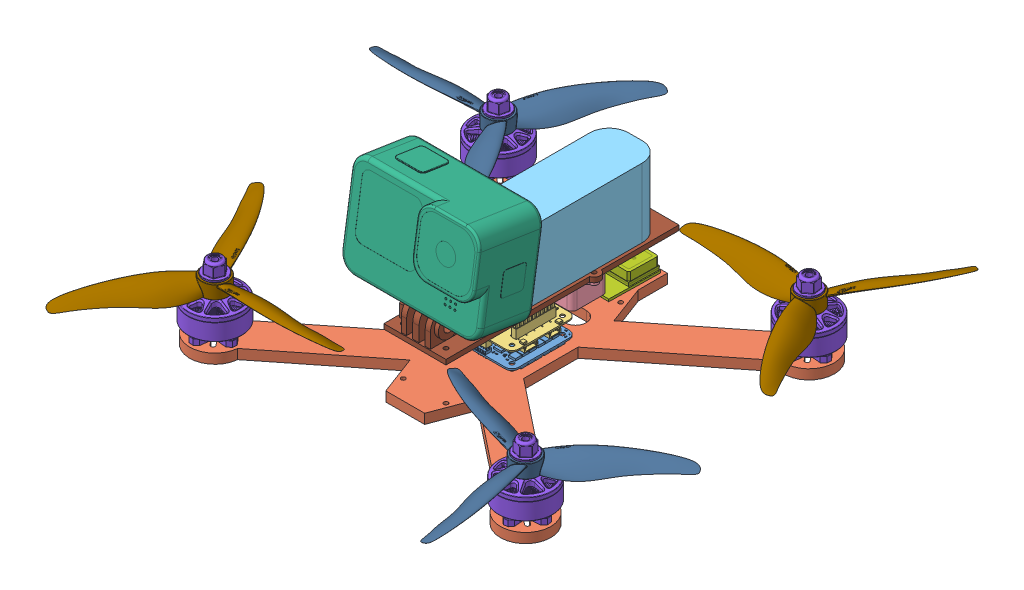
SolidWorks assembly Quad_assem, configuration Default. Lengths in mm.
Overall size (310.74 97.21 293.5).
16 component instances, 11 part files, 39 mates.
Components (placement in the parent):
- 4in1_ESC-1: 4in1_ESC [Default] at (-19.4317 7.836 116.374) x (-1 0 0) z (0 1 0) size (33 33 7.6)
- Quad-1: Quad [Default] at (-19.4317 0 116.374) x (-1 0 0) z (0 0 -1) size (186 5 172)
- FlightController.step-1: FlightController.step [Default] at (-19.4317 15.9597 116.374) x (-1 0 0) z (0 1 0) size (33 33 15.78)
- ToF-1: ToF [Default] at (-19.4317 27 89.374) x (1 0 0) z (0 0 -1) size (34.5 13.5 18.5)
- Battery-1: Battery [Default] at (-5 47.25 90.057) x (0 0 1) z (-1 0 0) size (72.6 35.5 27)
- GoPro Hero 9-1: GoPro Hero 9 [Default] at (-54.98 91.6448 135.3186) x (1 0 0) z (0 -0.98853 0.151026) size (72.1 33.6 50.5)
- GPS_sam-m8q-2: GPS_sam-m8q [Default] at (-27.0693 6.25 48.1086) x (0.999848 0 0.017452) z (-0.017452 0 0.999848) size (16.15 7.55 26.25)
- DYS SF2207 Motor.step-1: DYS SF2207 Motor.step [Default] at (60.5683 5 189.374) x (0.969016 0 -0.246999) z (0.246999 0 0.969016) size (27.7 33.34 27.7)
- DYS SF2207 Motor.step-2: DYS SF2207 Motor.step [Default] at (60.5683 5 43.374) x (0.997185 0 -0.074979) z (0.074979 0 0.997185) size (27.7 33.34 27.7)
- DYS SF2207 Motor.step-3: DYS SF2207 Motor.step [Default] at (-99.4317 5 43.374) x (0.246999 0 0.969016) z (-0.969016 0 0.246999) size (27.7 33.34 27.7)
- DYS SF2207 Motor.step-4: DYS SF2207 Motor.step [Default] at (-99.4317 5 189.374) x (0.074979 0 0.997185) z (-0.997185 0 0.074979) size (27.7 33.34 27.7)
- 50 Prop CW-1: 50 Prop CW [Default] at (60.5683 24.2 43.374) x (0.500095 0 -0.865971) z (0.865971 0 0.500095) size (98.6 8.5 111.89)
- 50 Prop CCW-1: 50 Prop CCW [Default] at (140.3677 27.725 231.543) x (-0.75515 0 0.655552) z (-0.655552 0 -0.75515) size (98.59 8.5 111.89)
- 50 Prop CCW-2: 50 Prop CCW [Default] at (-9.7231 27.725 53.3005) x (-0.461735 0 0.887018) z (-0.887018 0 -0.461735) size (98.59 8.5 111.89)
- 50 Prop CW-2: 50 Prop CW [Default] at (-99.4317 24.2 189.374) size (98.6 8.5 111.89)
- Quad Top-1: Quad Top [Default] at (-19.4317 27 116.374) x (-1 0 0) z (0 0 -1) size (36.7 17.5 120)
Mates (geometry in assembly coordinates):
- Concentric3: concentric aligned: circle of 4in1_ESC-1; circle of FlightController.step-1
- Concentric4: concentric aligned: circle of 4in1_ESC-1; circle of FlightController.step-1
- Distance3: distance = 7.5 mm anti-aligned: plane of 4in1_ESC-1 through (-2.9317 7.836 103.374) normal (0 1 0); plane of FlightController.step-1 through (-2.9317 15.336 103.374) normal (0 -1 0)
- Distance6: distance = 5 mm aligned: plane of Battery-1 through (-5 47.25 90.057) normal (1 0 0)
- Distance7: distance = 55 mm anti-aligned: plane of GoPro Hero 9-1 through (-55 91.6448 135.3186) normal (-1 0 0)
- Concentric5: concentric aligned: circle of 4in1_ESC-1; circle of Quad-1
- Concentric6: concentric aligned: circle of 4in1_ESC-1; circle of Quad-1
- Distance8: distance = 2 mm anti-aligned: plane of Quad-1 through (60.5683 5 189.374) normal (0 1 0); plane of 4in1_ESC-1 through (-2.9317 7 103.374) normal (0 -1 0)
- Coincident38: coincident anti-aligned: plane of Quad-1 through (60.5683 5 189.374) normal (0 1 0); plane of DYS SF2207 Motor.step-1 through (64.7816 5 192.9093) normal (0 -1 0)
- Concentric7: concentric aligned: circle of Quad-1; circle of DYS SF2207 Motor.step-1
- Concentric8: concentric aligned: circle of Quad-1; circle of DYS SF2207 Motor.step-1
- Coincident39: coincident anti-aligned: plane of Quad-1 through (60.5683 5 189.374) normal (0 1 0); plane of DYS SF2207 Motor.step-2 through (64.1036 5 47.5872) normal (0 -1 0)
- Coincident40: coincident anti-aligned: plane of Quad-1 through (60.5683 5 189.374) normal (0 1 0); plane of DYS SF2207 Motor.step-3 through (-102.967 5 47.5872) normal (0 -1 0)
- Coincident41: coincident anti-aligned: plane of Quad-1 through (60.5683 5 189.374) normal (0 1 0); plane of DYS SF2207 Motor.step-4 through (-103.6449 5 192.9093) normal (0 -1 0)
- Coincident42: coincident anti-aligned: plane of DYS SF2207 Motor.step-1 through (63.3364 24.2 184.8543) normal (0 1 0); plane of 50 Prop CCW-1 through (60.5683 24.2 189.374) normal (0 -1 0)
- Coincident43: coincident anti-aligned: plane of DYS SF2207 Motor.step-3 through (-94.912 24.2 46.142) normal (0 1 0); plane of 50 Prop CCW-2 through (-99.4317 24.2 43.374) normal (0 -1 0)
- Coincident44: coincident anti-aligned: plane of DYS SF2207 Motor.step-4 through (-95.4613 24.2 192.8848) normal (0 1 0); plane of 50 Prop CW-2 through (-99.4317 24.2 189.374) normal (0 -1 0)
- Coincident45: coincident anti-aligned: plane of DYS SF2207 Motor.step-2 through (64.0792 24.2 39.4036) normal (0 1 0); plane of 50 Prop CW-1 through (60.5683 24.2 43.374) normal (0 -1 0)
- Concentric15: concentric aligned: cylinder of DYS SF2207 Motor.step-1 through (60.5683 24.2 189.374) axis (0 1 0) radius 2.5; cylinder of 50 Prop CCW-1 through (60.5683 27.7 189.374) axis (0 1 0) radius 2.5
- Concentric16: concentric anti-aligned: cylinder of DYS SF2207 Motor.step-2 through (60.5683 24.2 43.374) axis (0 1 0) radius 2.5; cylinder of 50 Prop CW-1 through (60.5683 27.7 43.374) axis (0 -1 0) radius 2.5
- Concentric17: concentric aligned: cylinder of DYS SF2207 Motor.step-3 through (-99.4317 24.2 43.374) axis (0 1 0) radius 2.5; cylinder of 50 Prop CCW-2 through (-99.4317 27.7 43.374) axis (0 1 0) radius 2.5
- Concentric18: concentric anti-aligned: cylinder of DYS SF2207 Motor.step-4 through (-99.4317 24.2 189.374) axis (0 1 0) radius 2.5; cylinder of 50 Prop CW-2 through (-99.4317 27.7 189.374) axis (0 -1 0) radius 2.5
- Concentric19: concentric aligned: cylinder of DYS SF2207 Motor.step-3 through (-99.4317 24.2 43.374) axis (0 1 0) radius 2.5; cylinder of 50 Prop CCW-2 through (-99.4317 27.7 43.374) axis (0 1 0) radius 2.5
- Tangent1: tangent anti-aligned: plane of GoPro Hero 9-1 through (9.02 46.4018 170.2521) normal (0 -0.98853 0.151026); cylinder of Quad Top-1 through (-19.4317 37 158.374) axis (-1 0 0) radius 7.5
- Concentric23: concentric anti-aligned: circle of ToF-1; circle of Quad Top-1
- Concentric24: concentric anti-aligned: circle of ToF-1; circle of Quad Top-1
- Coincident53: coincident anti-aligned: plane of ToF-1 through (-8.7317 27 82.624) normal (0 1 0); plane of Quad Top-1 through (-4.1817 27 89.374) normal (0 -1 0)
- Concentric25: concentric aligned: circle of Quad-1; circle of Quad Top-1
- Concentric26: concentric aligned: circle of Quad-1; circle of Quad Top-1
- Coincident56: coincident anti-aligned: plane of Battery-1 through (-32 29.5 53.757) normal (0 -1 0); plane of Quad Top-1 through (-4.1817 29.5 89.374) normal (0 1 0)
- Concentric27: concentric aligned: circle of Quad-1; circle of DYS SF2207 Motor.step-2
- Concentric28: concentric aligned: circle of Quad-1; circle of DYS SF2207 Motor.step-2
- Concentric29: concentric aligned: circle of Quad-1; circle of DYS SF2207 Motor.step-3
- Concentric30: concentric aligned: circle of Quad-1; circle of DYS SF2207 Motor.step-3
- Concentric31: concentric aligned: circle of Quad-1; circle of DYS SF2207 Motor.step-4
- Concentric32: concentric aligned: circle of Quad-1; circle of DYS SF2207 Motor.step-4
- Coincident57: coincident anti-aligned: plane of Quad-1 through (60.5683 0 189.374) normal (0 -1 0)
- Coincident58: coincident anti-aligned: plane of Quad-1 through (60.5683 5 189.374) normal (0 1 0); plane of GPS_sam-m8q-2 through (-27.0693 5 48.1086) normal (0 -1 0)
- Distance9: distance = 22 mm anti-aligned: plane of Quad Top-1 through (-4.1817 27 89.374) normal (0 -1 0); plane of Quad-1 through (60.5683 5 189.374) normal (0 1 0)
